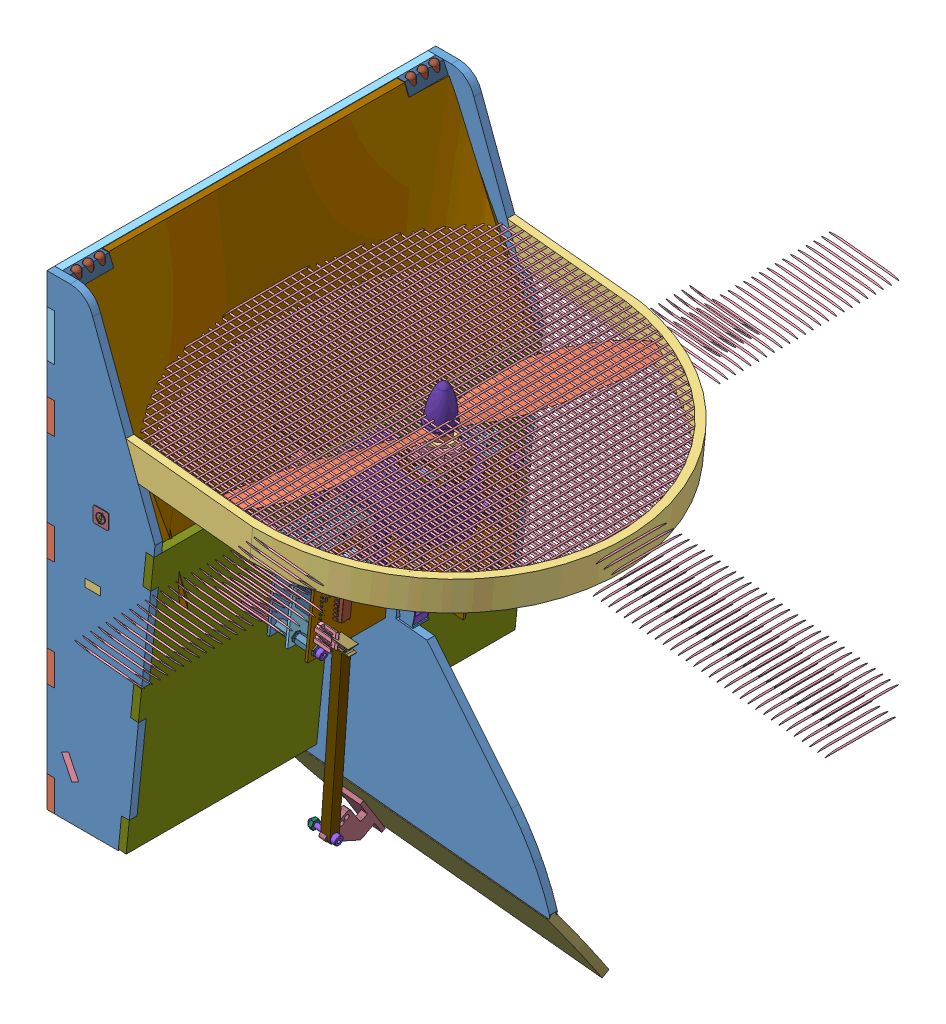
SolidWorks assembly AssTotaleSimu7, configuration Défaut. Lengths in mm.
Overall size (253.25 382.9 251.6).
1779 component instances, 238 part files, 11 mates.
Components (placement in the parent):
- AssStructSimu-1: AssStructSimu [Défaut] at (-125.7658 -1.8483 624.6548) x (1 0 0) z (0 0 -1) size (253.25 324.59 251.6)
  - AssBase-1: AssBase [Défaut] at (36.5482 -71.0398 34.0612) size (86.08 302.3 251.6)
    - AssD-1: AssD [Défaut] at (39.0992 31.0201 8.5) size (69.5 300 22)
      - P1-1: P1 [Défaut] at (-95.5819 194.6656 377.5) size (69.5 300 5)
      - P5-1: P5 [Défaut] at (-100.5819 -35.3344 360.5) x (0 1 0) z (1 0 0) size (230 22 5)
    - AssG-1: AssG [Défaut] at (39.0992 31.0201 -236.5) size (69.5 300 22)
      - P1-1: P1 [Défaut] at (-95.5819 194.6656 377.5) size (69.5 300 5)
      - P5-1: P5 [Défaut] at (-95.5819 -35.3344 399.5) x (0 1 0) z (-1 0 0) size (230 22 5)
    - P7-1: P7 [Défaut] at (-1.4828 89.6857 370.5) x (0 0 -1) z (0 -1 0) size (250 54.5 5)
    - P4-1: P4 [Défaut] at (-63.2363 165.9323 386) x (0 0 -1) z (0.898794 -0.438371 0) size (250 60.5 66.27)
    - P3-1: P3 [Défaut] at (-56.4828 -74.3143 146) x (0 0 1) z (-1 0 0) size (250 70 5)
    - P4b-1: P4b [Défaut] at (-58.7423 163.7404 190) x (0 0 1) z (0.438371 0.898794 0) size (152 56 2)
    - battery-1: battery [Défaut] at (-39.0156 204.1861 197.5) x (0 0 1) z (0.898794 -0.438371 0) size (137 43 30)
    - socket head cap screw 4762_din-1: socket head cap screw 4762_din [EN ISO 4762 M3 x 10 - 10N] at (-27.7008 145.2627 193) x (0.438371 0.898794 0) z (0 0 -1) size (13 5.5 5.5)
    - socket head cap screw 4762_din-2: socket head cap screw 4762_din [EN ISO 4762 M3 x 10 - 10N] at (-27.7008 145.2627 339) x (0.438371 0.898794 0) z (-0.791285 0.385936 -0.474259) size (13 5.5 5.5)
    - socket head cap screw 4762_din-3: socket head cap screw 4762_din [EN ISO 4762 M3 x 10 - 10N] at (-42.0815 152.2766 339) x (0.438371 0.898794 0) z (-0.001489 0.000726 -0.999999) size (13 5.5 5.5)
    - socket head cap screw 4762_din-4: socket head cap screw 4762_din [EN ISO 4762 M3 x 10 - 10N] at (-42.0815 152.2766 193) x (0.438371 0.898794 0) z (-0.031331 0.015281 -0.999392) size (13 5.5 5.5)
    - P11-1: P11 [Défaut] at (-57.5734 -73.9703 146.7843) x (0.005072 0 0.999987) z (0.006197 0.999981 -0.000031) size (240 65 164)
    - AssPhare-1: AssPhare [Défaut] at (-52.8518 -67.6977 411) x (0 1 0) z (0 0 -1) size (35.8 8 25)
      - piece_led-1: piece_led [Défaut] at (-6.6166 -3.631 25) size (7 8 25)
      - LED 5mm-1: LED 5mm [Valor predeterminado] at (-0.1166 0.369 30) x (0 0 1) z (-1 0 0) size (10.06 6 40.8)
      - LED 5mm-2: LED 5mm [Valor predeterminado] at (-0.1166 0.369 37.5) x (0 0 1) z (-1 0 0) size (10.06 6 40.8)
      - LED 5mm-3: LED 5mm [Valor predeterminado] at (-0.1166 0.369 45) x (0 0 1) z (-1 0 0) size (10.06 6 40.8)
    - AssPhare-2: AssPhare [Défaut] at (-52.8518 -67.6977 196) x (0 1 0) z (0 0 -1) size (35.8 8 25)
      - piece_led-1: piece_led [Défaut] at (-6.6166 -3.631 25) size (7 8 25)
      - LED 5mm-1: LED 5mm [Valor predeterminado] at (-0.1166 0.369 30) x (0 0 1) z (-1 0 0) size (10.06 6 40.8)
      - LED 5mm-2: LED 5mm [Valor predeterminado] at (-0.1166 0.369 37.5) x (0 0 1) z (-1 0 0) size (10.06 6 40.8)
      - LED 5mm-3: LED 5mm [Valor predeterminado] at (-0.1166 0.369 45) x (0 0 1) z (-1 0 0) size (10.06 6 40.8)
    - AssLogo-1: AssLogo [Défaut] at (-27.8835 45.1673 148.1054) x (-1 0 0) z (0 0 -1) size (10 10 0.8)
      - logo1-1: logo1 [Défaut] at (-6.5271 -4.4734 6.5054) size (5.8 7.71 0.4)
      - logo2-1: logo2 [Défaut] at (-6.4007 -4.4815 7.1054) size (10 10 0.4)
    - AssLogo-2: AssLogo [Défaut] at (-25.082 45.1673 383.8946) size (10 10 0.8)
      - logo1-1: logo1 [Défaut] at (-6.5271 -4.4734 6.5054) size (5.8 7.71 0.4)
      - logo2-1: logo2 [Défaut] at (-6.4007 -4.4815 7.1054) size (10 10 0.4)
    - support2-1: support2 [Défaut] at (-61.5648 191.7124 276) x (-0.017452 -0.999848 0) z (0.999848 -0.017452 0) size (75 20 10)
    - socket head cap screw 4762_din-5: socket head cap screw 4762_din [EN ISO 4762 M3 x 5 - 5N] at (-61.652 186.7132 269.3333) x (0.999848 -0.017452 0) z (-0.002158 -0.123615 0.992328) size (8 5.5 5.5)
    - socket head cap screw 4762_din-6: socket head cap screw 4762_din [EN ISO 4762 M3 x 5 - 5N] at (-61.652 186.7132 262.6667) x (0.999848 -0.017452 0) z (0 0 1) size (8 5.5 5.5)
    - socket head cap screw 4762_din-7: socket head cap screw 4762_din [EN ISO 4762 M3 x 25 - 18N] at (-55.2963 121.0922 253) x (0 0 1) z (-1 0 0) size (28 5.5 5.5)
    - hex nut style 1 gradeab_din-1: hex nut style 1 gradeab_din [Hexagon Nut ISO 4032 - M3 - W - N] at (-55.2963 121.0922 276) x (-0.923728 -0.383049 0) z (0 0 -1) size (5.5 6.35 2.4)
  - AssToitMot-1: AssToitMot [Défaut] at (-168.5238 43.6961 238.494) x (0 0 -1) z (0.9948 0.101852 0) size (250 207.5 205)
    - AssToit-1: AssToit [Défaut] at (-23.0702 -16.5789 -3.7148) size (250 207.5 205)
      - P8-1: P8 [Défaut] at (-38.4971 122.5921 203.5) size (250 175 5)
      - P12-1: P12 [Défaut] at (-60.4971 -63.4079 265.5) x (1 0 0) z (0 -1 0) size (44.28 76.64 55)
      - P13-1: P13 [Défaut] at (-35.9971 -52.8579 208.5) x (0 0 1) z (-1 0 0) size (64 15.55 5)
      - P10_2-1: P10_2 [Défaut] at (-35.9971 111.5921 171) x (0 0 1) z (-1 0 0) size (188.5 117.6 5)
    - Parallax-Servo_DUMMY-1: Parallax-Servo_DUMMY [Défaut] at (-61.6002 -51.5207 216.6662) x (1 0 0) z (0 1 0) size (20.07 42.67 55.64)
    - socket head cap screw 4762_din-1: socket head cap screw 4762_din [EN ISO 4762 M2.5 x 5 - 5N] at (-51.9272 -76.4868 259.2852) x (0 -1 0) z (-0.546944 0 0.837169) size (7.5 4.5 4.5)
    - socket head cap screw 4762_din-2: socket head cap screw 4762_din [EN ISO 4762 M2.5 x 5 - 5N] at (-61.5672 -76.4868 268.9252) x (0 -1 0) z (-0.546944 0 0.837169) size (7.5 4.5 4.5)
    - socket head cap screw 4762_din-3: socket head cap screw 4762_din [EN ISO 4762 M2.5 x 5 - 5N] at (-71.2072 -76.4868 259.2852) x (0 -1 0) z (-0.546944 0 0.837169) size (7.5 4.5 4.5)
    - socket head cap screw 4762_din-4: socket head cap screw 4762_din [EN ISO 4762 M2.5 x 5 - 5N] at (-61.5672 -76.4868 249.6452) x (0 -1 0) z (-0.546944 0 0.837169) size (7.5 4.5 4.5)
    - AssPhare-1: AssPhare [Défaut] at (8.4328 83.3966 196.1542) x (0 -1 0) z (1 0 0) size (35.8 8 25)
      - piece_led-1: piece_led [Défaut] at (-6.6166 -3.631 25) size (7 8 25)
      - LED 5mm-1: LED 5mm [Valor predeterminado] at (-0.1166 0.369 30) x (0 0 1) z (-1 0 0) size (10.06 6 40.8)
      - LED 5mm-2: LED 5mm [Valor predeterminado] at (-0.1166 0.369 37.5) x (0 0 1) z (-1 0 0) size (10.06 6 40.8)
      - LED 5mm-3: LED 5mm [Valor predeterminado] at (-0.1166 0.369 45) x (0 0 1) z (-1 0 0) size (10.06 6 40.8)
    - AssPhare-2: AssPhare [Défaut] at (-206.5672 83.3966 196.1542) x (0 -1 0) z (1 0 0) size (35.8 8 25)
      - piece_led-1: piece_led [Défaut] at (-6.6166 -3.631 25) size (7 8 25)
      - LED 5mm-1: LED 5mm [Valor predeterminado] at (-0.1166 0.369 30) x (0 0 1) z (-1 0 0) size (10.06 6 40.8)
      - LED 5mm-2: LED 5mm [Valor predeterminado] at (-0.1166 0.369 37.5) x (0 0 1) z (-1 0 0) size (10.06 6 40.8)
      - LED 5mm-3: LED 5mm [Valor predeterminado] at (-0.1166 0.369 45) x (0 0 1) z (-1 0 0) size (10.06 6 40.8)
    - socket head cap screw 4762_din-5: socket head cap screw 4762_din [EN ISO 4762 M3 x 10 - 10N] at (-67.0672 -22.9368 210.2852) x (0 0 -1) z (1 0 0) size (13 5.5 5.5)
    - socket head cap screw 4762_din-6: socket head cap screw 4762_din [EN ISO 4762 M3 x 10 - 10N] at (-56.0672 -72.9868 210.2852) x (0 0 -1) z (1 0 0) size (13 5.5 5.5)
    - socket head cap screw 4762_din-7: socket head cap screw 4762_din [EN ISO 4762 M3 x 10 - 10N] at (-67.0672 -72.9868 210.2852) x (0 0 -1) z (1 0 0) size (13 5.5 5.5)
    - socket head cap screw 4762_din-8: socket head cap screw 4762_din [EN ISO 4762 M3 x 10 - 10N] at (-56.0672 -22.9368 210.2852) x (0 0 -1) z (1 0 0) size (13 5.5 5.5)
    - hex nut style 1 gradeab_din-1: hex nut style 1 gradeab_din [Hexagon Nut ISO 4032 - M3 - W - N] at (-67.0672 -72.9868 197.3852) x (-0.923728 -0.383049 0) z (0 0 -1) size (5.5 6.35 2.4)
    - hex nut style 1 gradeab_din-2: hex nut style 1 gradeab_din [Hexagon Nut ISO 4032 - M3 - W - N] at (-56.0672 -72.9868 199.7852) size (5.5 6.35 2.4)
    - hex nut style 1 gradeab_din-3: hex nut style 1 gradeab_din [Hexagon Nut ISO 4032 - M3 - W - N] at (-67.0672 -22.9368 199.7852) size (5.5 6.35 2.4)
    - hex nut style 1 gradeab_din-4: hex nut style 1 gradeab_din [Hexagon Nut ISO 4032 - M3 - W - N] at (-56.0672 -22.9368 199.7852) size (5.5 6.35 2.4)
  - AssProtec-1: AssProtec [Défaut] at (86.6746 190.4649 284.6351) x (0 0 -1) z (0.101852 -0.9948 0) size (250 237.46 20)
    - protec3c-1: protec3c [Défaut] at (-140.4261 -87.7568 240) size (250 197 20)
    - AssGrillage-1: AssGrillage [Défaut] at (-370.4609 -132.5428 258.3161) x (0 0 -1) z (1 0 0) size (2.02 237.05 250)
      - barreau-1: barreau [Défaut] at (-1.1839 0.254 200) size (1 1 400)
      - barreau-3: barreau [Défaut] at (-1.1839 5.254 200) size (1 1 400)
      - barreau-4: barreau [Défaut] at (-1.1839 10.254 200) size (1 1 400)
      - barreau-5: barreau [Défaut] at (-1.1839 15.254 200) size (1 1 400)
      - barreau-6: barreau [Défaut] at (-1.1839 20.254 200) size (1 1 400)
      - barreau-7: barreau [Défaut] at (-1.1839 25.254 200) size (1 1 400)
      - barreau-8: barreau [Défaut] at (-1.1839 30.254 200) size (1 1 400)
      - barreau-9: barreau [Défaut] at (-1.1839 35.254 200) size (1 1 400)
      - barreau-10: barreau [Défaut] at (-1.1839 40.254 200) size (1 1 400)
      - barreau-11: barreau [Défaut] at (-1.1839 45.254 200) size (1 1 400)
      - barreau-12: barreau [Défaut] at (-1.1839 50.254 200) size (1 1 400)
      - barreau-13: barreau [Défaut] at (-1.1839 55.254 200) size (1 1 400)
      - barreau-14: barreau [Défaut] at (-1.1839 60.254 200) size (1 1 400)
      - barreau-15: barreau [Défaut] at (-1.1839 65.254 200) size (1 1 400)
      - barreau-16: barreau [Défaut] at (-1.1839 70.254 200) size (1 1 400)
      - barreau-17: barreau [Défaut] at (-1.1839 75.254 200) size (1 1 400)
      - barreau-18: barreau [Défaut] at (-1.1839 80.254 200) size (1 1 400)
      - barreau-19: barreau [Défaut] at (-1.1839 85.254 200) size (1 1 400)
      - barreau-20: barreau [Défaut] at (-1.1839 90.254 200) size (1 1 400)
      - barreau-21: barreau [Défaut] at (-1.1839 95.254 200) size (1 1 400)
      - barreau-22: barreau [Défaut] at (-1.1839 100.254 200) size (1 1 400)
      - barreau-23: barreau [Défaut] at (-1.1839 105.254 200) size (1 1 400)
      - barreau-24: barreau [Défaut] at (-1.1839 110.254 200) size (1 1 400)
      - barreau-25: barreau [Défaut] at (-1.1839 115.254 200) size (1 1 400)
      - barreau-26: barreau [Défaut] at (-1.1839 120.254 200) size (1 1 400)
      - barreau-27: barreau [Défaut] at (-1.1839 125.254 200) size (1 1 400)
      - barreau-28: barreau [Défaut] at (-1.1839 130.254 200) size (1 1 400)
      - barreau-29: barreau [Défaut] at (-1.1839 135.254 200) size (1 1 400)
      - barreau-30: barreau [Défaut] at (-1.1839 140.254 200) size (1 1 400)
      - barreau-31: barreau [Défaut] at (-1.1839 145.254 200) size (1 1 400)
      - barreau-32: barreau [Défaut] at (-1.1839 150.254 200) size (1 1 400)
      - barreau-33: barreau [Défaut] at (-1.1839 155.254 200) size (1 1 400)
      - barreau-34: barreau [Défaut] at (-1.1839 160.254 200) size (1 1 400)
      - barreau-35: barreau [Défaut] at (-1.1839 165.254 200) size (1 1 400)
      - barreau-36: barreau [Défaut] at (-1.1839 170.254 200) size (1 1 400)
      - barreau-37: barreau [Défaut] at (-1.1839 175.254 200) size (1 1 400)
      - barreau-38: barreau [Défaut] at (-1.1839 180.254 200) size (1 1 400)
      - barreau-39: barreau [Défaut] at (-1.1839 185.254 200) size (1 1 400)
      - barreau-40: barreau [Défaut] at (-1.1839 190.254 200) size (1 1 400)
      - barreau-41: barreau [Défaut] at (-1.1839 195.254 200) size (1 1 400)
      - barreau-42: barreau [Défaut] at (-0.1839 -1.5314 598.7823) x (0.998922 0 0.04641) z (0 1 0) size (1 1 400)
      - barreau-43: barreau [Défaut] at (-1.1839 200.254 200) size (1 1 400)
      - barreau-44: barreau [Défaut] at (-1.1839 205.254 200) size (1 1 400)
      - barreau-45: barreau [Défaut] at (-1.1839 210.254 200) size (1 1 400)
      - barreau-46: barreau [Défaut] at (-1.1839 215.254 200) size (1 1 400)
      - barreau-47: barreau [Défaut] at (-1.1839 220.254 200) size (1 1 400)
      - barreau-48: barreau [Défaut] at (-1.1839 225.254 200) size (1 1 400)
      - barreau-49: barreau [Défaut] at (-1.1839 230.254 200) size (1 1 400)
      - barreau-50: barreau [Défaut] at (-1.1839 235.254 200) size (1 1 400)
      - barreau-51: barreau [Défaut] at (-1.1839 240.254 200) size (1 1 400)
      - barreau-52: barreau [Défaut] at (-1.1839 245.254 200) size (1 1 400)
      - barreau-53: barreau [Défaut] at (-1.1839 250.254 200) size (1 1 400)
      - barreau-54: barreau [Défaut] at (-1.1839 255.254 200) size (1 1 400)
      - barreau-55: barreau [Défaut] at (-1.1839 260.254 200) size (1 1 400)
      - barreau-56: barreau [Défaut] at (-1.1839 265.254 200) size (1 1 400)
      - barreau-57: barreau [Défaut] at (-1.1839 270.254 200) size (1 1 400)
      - barreau-58: barreau [Défaut] at (-1.1839 275.254 200) size (1 1 400)
      - barreau-59: barreau [Défaut] at (-1.1839 280.254 200) size (1 1 400)
      - barreau-60: barreau [Défaut] at (-1.1839 285.254 200) size (1 1 400)
      - barreau-61: barreau [Défaut] at (-1.1839 290.254 200) size (1 1 400)
      - barreau-62: barreau [Défaut] at (-1.1839 295.254 200) size (1 1 400)
      - barreau-63: barreau [Défaut] at (-1.1839 300.254 200) size (1 1 400)
      - barreau-64: barreau [Défaut] at (-1.1839 305.254 200) size (1 1 400)
      - barreau-65: barreau [Défaut] at (-1.1839 310.254 200) size (1 1 400)
      - barreau-66: barreau [Défaut] at (-1.1839 315.254 200) size (1 1 400)
      - barreau-67: barreau [Défaut] at (-1.1839 320.254 200) size (1 1 400)
      - barreau-68: barreau [Défaut] at (-1.1839 325.254 200) size (1 1 400)
      - barreau-69: barreau [Défaut] at (-1.1839 330.254 200) size (1 1 400)
      - barreau-70: barreau [Défaut] at (-1.1839 335.254 200) size (1 1 400)
      - barreau-71: barreau [Défaut] at (-1.1839 340.254 200) size (1 1 400)
      - barreau-72: barreau [Défaut] at (-1.1839 345.254 200) size (1 1 400)
      - barreau-73: barreau [Défaut] at (-1.1839 350.254 200) size (1 1 400)
      - barreau-74: barreau [Défaut] at (-1.1839 355.254 200) size (1 1 400)
      - barreau-75: barreau [Défaut] at (-1.1839 360.254 200) size (1 1 400)
      - barreau-76: barreau [Défaut] at (-1.1839 365.254 200) size (1 1 400)
      - barreau-77: barreau [Défaut] at (-1.1839 370.254 200) size (1 1 400)
      - barreau-78: barreau [Défaut] at (-1.1839 375.254 200) size (1 1 400)
      - barreau-79: barreau [Défaut] at (-1.1839 380.254 200) size (1 1 400)
      - barreau-80: barreau [Défaut] at (-1.1839 385.254 200) size (1 1 400)
      - barreau-81: barreau [Défaut] at (-1.1839 390.254 200) size (1 1 400)
      - barreau-82: barreau [Défaut] at (-1.1839 395.254 200) size (1 1 400)
      - barreau-136: barreau [Défaut] at (-0.1839 -1.5314 593.7823) x (0.998922 0 0.04641) z (0 1 0) size (1 1 400)
      - barreau-137: barreau [Défaut] at (-0.1839 -1.5314 588.7823) x (0.998922 0 0.04641) z (0 1 0) size (1 1 400)
      - barreau-138: barreau [Défaut] at (-0.1839 -1.5314 583.7823) x (0.998922 0 0.04641) z (0 1 0) size (1 1 400)
      - barreau-139: barreau [Défaut] at (-0.1839 -1.5314 578.7823) x (0.998922 0 0.04641) z (0 1 0) size (1 1 400)
      - barreau-140: barreau [Défaut] at (-0.1839 -1.5314 573.7823) x (0.998922 0 0.04641) z (0 1 0) size (1 1 400)
      - barreau-141: barreau [Défaut] at (-0.1839 -1.5314 568.7823) x (0.998922 0 0.04641) z (0 1 0) size (1 1 400)
      - barreau-142: barreau [Défaut] at (-0.1839 -1.5314 563.7823) x (0.998922 0 0.04641) z (0 1 0) size (1 1 400)
      - barreau-143: barreau [Défaut] at (-0.1839 -1.5314 558.7823) x (0.998922 0 0.04641) z (0 1 0) size (1 1 400)
      - barreau-144: barreau [Défaut] at (-0.1839 -1.5314 553.7823) x (0.998922 0 0.04641) z (0 1 0) size (1 1 400)
      - barreau-145: barreau [Défaut] at (-0.1839 -1.5314 548.7823) x (0.998922 0 0.04641) z (0 1 0) size (1 1 400)
      - barreau-146: barreau [Défaut] at (-0.1839 -1.5314 543.7823) x (0.998922 0 0.04641) z (0 1 0) size (1 1 400)
      - barreau-147: barreau [Défaut] at (-0.1839 -1.5314 538.7823) x (0.998922 0 0.04641) z (0 1 0) size (1 1 400)
      - barreau-148: barreau [Défaut] at (-0.1839 -1.5314 533.7823) x (0.998922 0 0.04641) z (0 1 0) size (1 1 400)
      - barreau-149: barreau [Défaut] at (-0.1839 -1.5314 528.7823) x (0.998922 0 0.04641) z (0 1 0) size (1 1 400)
      - barreau-150: barreau [Défaut] at (-0.1839 -1.5314 523.7823) x (0.998922 0 0.04641) z (0 1 0) size (1 1 400)
      - barreau-151: barreau [Défaut] at (-0.1839 -1.5314 518.7823) x (0.998922 0 0.04641) z (0 1 0) size (1 1 400)
      - barreau-152: barreau [Défaut] at (-0.1839 -1.5314 513.7823) x (0.998922 0 0.04641) z (0 1 0) size (1 1 400)
      - barreau-153: barreau [Défaut] at (-0.1839 -1.5314 508.7823) x (0.998922 0 0.04641) z (0 1 0) size (1 1 400)
      - barreau-154: barreau [Défaut] at (-0.1839 -1.5314 503.7823) x (0.998922 0 0.04641) z (0 1 0) size (1 1 400)
      - barreau-155: barreau [Défaut] at (-0.1839 -1.5314 498.7823) x (0.998922 0 0.04641) z (0 1 0) size (1 1 400)
      - barreau-156: barreau [Défaut] at (-0.1839 -1.5314 493.7823) x (0.998922 0 0.04641) z (0 1 0) size (1 1 400)
      - barreau-157: barreau [Défaut] at (-0.1839 -1.5314 488.7823) x (0.998922 0 0.04641) z (0 1 0) size (1 1 400)
      - barreau-158: barreau [Défaut] at (-0.1839 -1.5314 483.7823) x (0.998922 0 0.04641) z (0 1 0) size (1 1 400)
      - barreau-159: barreau [Défaut] at (-0.1839 -1.5314 478.7823) x (0.998922 0 0.04641) z (0 1 0) size (1 1 400)
      - barreau-160: barreau [Défaut] at (-0.1839 -1.5314 473.7823) x (0.998922 0 0.04641) z (0 1 0) size (1 1 400)
      - barreau-161: barreau [Défaut] at (-0.1839 -1.5314 468.7823) x (0.998922 0 0.04641) z (0 1 0) size (1 1 400)
      - barreau-162: barreau [Défaut] at (-0.1839 -1.5314 463.7823) x (0.998922 0 0.04641) z (0 1 0) size (1 1 400)
      - barreau-163: barreau [Défaut] at (-0.1839 -1.5314 458.7823) x (0.998922 0 0.04641) z (0 1 0) size (1 1 400)
      - barreau-164: barreau [Défaut] at (-0.1839 -1.5314 453.7823) x (0.998922 0 0.04641) z (0 1 0) size (1 1 400)
      - barreau-165: barreau [Défaut] at (-0.1839 -1.5314 448.7823) x (0.998922 0 0.04641) z (0 1 0) size (1 1 400)
      - barreau-166: barreau [Défaut] at (-0.1839 -1.5314 443.7823) x (0.998922 0 0.04641) z (0 1 0) size (1 1 400)
      - barreau-167: barreau [Défaut] at (-0.1839 -1.5314 438.7823) x (0.998922 0 0.04641) z (0 1 0) size (1 1 400)
      - barreau-168: barreau [Défaut] at (-0.1839 -1.5314 433.7823) x (0.998922 0 0.04641) z (0 1 0) size (1 1 400)
      - barreau-169: barreau [Défaut] at (-0.1839 -1.5314 428.7823) x (0.998922 0 0.04641) z (0 1 0) size (1 1 400)
      - barreau-170: barreau [Défaut] at (-0.1839 -1.5314 423.7823) x (0.998922 0 0.04641) z (0 1 0) size (1 1 400)
      - barreau-171: barreau [Défaut] at (-0.1839 -1.5314 418.7823) x (0.998922 0 0.04641) z (0 1 0) size (1 1 400)
      - barreau-172: barreau [Défaut] at (-0.1839 -1.5314 413.7823) x (0.998922 0 0.04641) z (0 1 0) size (1 1 400)
      - barreau-173: barreau [Défaut] at (-0.1839 -1.5314 408.7823) x (0.998922 0 0.04641) z (0 1 0) size (1 1 400)
      - barreau-174: barreau [Défaut] at (-0.1839 -1.5314 403.7823) x (0.998922 0 0.04641) z (0 1 0) size (1 1 400)
      - barreau-175: barreau [Défaut] at (-0.1839 -1.5314 398.7823) x (0.998922 0 0.04641) z (0 1 0) size (1 1 400)
      - barreau-176: barreau [Défaut] at (-0.1839 -1.5314 393.7823) x (0.998922 0 0.04641) z (0 1 0) size (1 1 400)
      - barreau-177: barreau [Défaut] at (-0.1839 -1.5314 388.7823) x (0.998922 0 0.04641) z (0 1 0) size (1 1 400)
      - barreau-178: barreau [Défaut] at (-0.1839 -1.5314 383.7823) x (0.998922 0 0.04641) z (0 1 0) size (1 1 400)
      - barreau-179: barreau [Défaut] at (-0.1839 -1.5314 378.7823) x (0.998922 0 0.04641) z (0 1 0) size (1 1 400)
      - barreau-180: barreau [Défaut] at (-0.1839 -1.5314 373.7823) x (0.998922 0 0.04641) z (0 1 0) size (1 1 400)
      - barreau-181: barreau [Défaut] at (-0.1839 -1.5314 368.7823) x (0.998922 0 0.04641) z (0 1 0) size (1 1 400)
      - barreau-182: barreau [Défaut] at (-0.1839 -1.5314 363.7823) x (0.998922 0 0.04641) z (0 1 0) size (1 1 400)
      - barreau-183: barreau [Défaut] at (-0.1839 -1.5314 358.7823) x (0.998922 0 0.04641) z (0 1 0) size (1 1 400)
      - barreau-184: barreau [Défaut] at (-0.1839 -1.5314 353.7823) x (0.998922 0 0.04641) z (0 1 0) size (1 1 400)
      - barreau-185: barreau [Défaut] at (-0.1839 -1.5314 348.7823) x (0.998922 0 0.04641) z (0 1 0) size (1 1 400)
      - barreau-186: barreau [Défaut] at (-0.1839 -1.5314 343.7823) x (0.998922 0 0.04641) z (0 1 0) size (1 1 400)
      - barreau-187: barreau [Défaut] at (-0.1839 -1.5314 338.7823) x (0.998922 0 0.04641) z (0 1 0) size (1 1 400)
      - barreau-188: barreau [Défaut] at (-0.1839 -1.5314 333.7823) x (0.998922 0 0.04641) z (0 1 0) size (1 1 400)
      - barreau-189: barreau [Défaut] at (-0.1839 -1.5314 328.7823) x (0.998922 0 0.04641) z (0 1 0) size (1 1 400)
      - barreau-190: barreau [Défaut] at (-0.1839 -1.5314 323.7823) x (0.998922 0 0.04641) z (0 1 0) size (1 1 400)
      - barreau-191: barreau [Défaut] at (-0.1839 -1.5314 318.7823) x (0.998922 0 0.04641) z (0 1 0) size (1 1 400)
      - barreau-192: barreau [Défaut] at (-0.1839 -1.5314 313.7823) x (0.998922 0 0.04641) z (0 1 0) size (1 1 400)
      - barreau-193: barreau [Défaut] at (-0.1839 -1.5314 308.7823) x (0.998922 0 0.04641) z (0 1 0) size (1 1 400)
      - barreau-194: barreau [Défaut] at (-0.1839 -1.5314 303.7823) x (0.998922 0 0.04641) z (0 1 0) size (1 1 400)
      - barreau-195: barreau [Défaut] at (-0.1839 -1.5314 298.7823) x (0.998922 0 0.04641) z (0 1 0) size (1 1 400)
      - barreau-196: barreau [Défaut] at (-0.1839 -1.5314 293.7823) x (0.998922 0 0.04641) z (0 1 0) size (1 1 400)
      - barreau-197: barreau [Défaut] at (-0.1839 -1.5314 288.7823) x (0.998922 0 0.04641) z (0 1 0) size (1 1 400)
      - barreau-198: barreau [Défaut] at (-0.1839 -1.5314 283.7823) x (0.998922 0 0.04641) z (0 1 0) size (1 1 400)
      - barreau-199: barreau [Défaut] at (-0.1839 -1.5314 278.7823) x (0.998922 0 0.04641) z (0 1 0) size (1 1 400)
      - barreau-200: barreau [Défaut] at (-0.1839 -1.5314 273.7823) x (0.998922 0 0.04641) z (0 1 0) size (1 1 400)
      - barreau-201: barreau [Défaut] at (-0.1839 -1.5314 268.7823) x (0.998922 0 0.04641) z (0 1 0) size (1 1 400)
      - barreau-202: barreau [Défaut] at (-0.1839 -1.5314 263.7823) x (0.998922 0 0.04641) z (0 1 0) size (1 1 400)
      - barreau-203: barreau [Défaut] at (-0.1839 -1.5314 258.7823) x (0.998922 0 0.04641) z (0 1 0) size (1 1 400)
      - barreau-204: barreau [Défaut] at (-0.1839 -1.5314 253.7823) x (0.998922 0 0.04641) z (0 1 0) size (1 1 400)
      - barreau-205: barreau [Défaut] at (-0.1839 -1.5314 248.7823) x (0.998922 0 0.04641) z (0 1 0) size (1 1 400)
      - barreau-206: barreau [Défaut] at (-0.1839 -1.5314 243.7823) x (0.998922 0 0.04641) z (0 1 0) size (1 1 400)
      - barreau-207: barreau [Défaut] at (-0.1839 -1.5314 238.7823) x (0.998922 0 0.04641) z (0 1 0) size (1 1 400)
      - barreau-208: barreau [Défaut] at (-0.1839 -1.5314 233.7823) x (0.998922 0 0.04641) z (0 1 0) size (1 1 400)
      - barreau-209: barreau [Défaut] at (-0.1839 -1.5314 228.7823) x (0.998922 0 0.04641) z (0 1 0) size (1 1 400)
      - barreau-210: barreau [Défaut] at (-0.1839 -1.5314 223.7823) x (0.998922 0 0.04641) z (0 1 0) size (1 1 400)
      - barreau-211: barreau [Défaut] at (-0.1839 -1.5314 218.7823) x (0.998922 0 0.04641) z (0 1 0) size (1 1 400)
      - barreau-212: barreau [Défaut] at (-0.1839 -1.5314 213.7823) x (0.998922 0 0.04641) z (0 1 0) size (1 1 400)
      - barreau-213: barreau [Défaut] at (-0.1839 -1.5314 208.7823) x (0.998922 0 0.04641) z (0 1 0) size (1 1 400)
      - barreau-214: barreau [Défaut] at (-0.1839 -1.5314 203.7823) x (0.998922 0 0.04641) z (0 1 0) size (1 1 400)
    - AssGrillage-2: AssGrillage [Défaut] at (339.6086 -132.5428 241.6839) x (0 0 1) z (-1 0 0) size (2.02 237.05 250)
      - barreau-1: barreau [Défaut] at (-1.1839 0.254 200) size (1 1 400)
      - barreau-3: barreau [Défaut] at (-1.1839 5.254 200) size (1 1 400)
      - barreau-4: barreau [Défaut] at (-1.1839 10.254 200) size (1 1 400)
      - barreau-5: barreau [Défaut] at (-1.1839 15.254 200) size (1 1 400)
      - barreau-6: barreau [Défaut] at (-1.1839 20.254 200) size (1 1 400)
      - barreau-7: barreau [Défaut] at (-1.1839 25.254 200) size (1 1 400)
      - barreau-8: barreau [Défaut] at (-1.1839 30.254 200) size (1 1 400)
      - barreau-9: barreau [Défaut] at (-1.1839 35.254 200) size (1 1 400)
      - barreau-10: barreau [Défaut] at (-1.1839 40.254 200) size (1 1 400)
      - barreau-11: barreau [Défaut] at (-1.1839 45.254 200) size (1 1 400)
      - barreau-12: barreau [Défaut] at (-1.1839 50.254 200) size (1 1 400)
      - barreau-13: barreau [Défaut] at (-1.1839 55.254 200) size (1 1 400)
      - barreau-14: barreau [Défaut] at (-1.1839 60.254 200) size (1 1 400)
      - barreau-15: barreau [Défaut] at (-1.1839 65.254 200) size (1 1 400)
      - barreau-16: barreau [Défaut] at (-1.1839 70.254 200) size (1 1 400)
      - barreau-17: barreau [Défaut] at (-1.1839 75.254 200) size (1 1 400)
      - barreau-18: barreau [Défaut] at (-1.1839 80.254 200) size (1 1 400)
      - barreau-19: barreau [Défaut] at (-1.1839 85.254 200) size (1 1 400)
      - barreau-20: barreau [Défaut] at (-1.1839 90.254 200) size (1 1 400)
      - barreau-21: barreau [Défaut] at (-1.1839 95.254 200) size (1 1 400)
      - barreau-22: barreau [Défaut] at (-1.1839 100.254 200) size (1 1 400)
      - barreau-23: barreau [Défaut] at (-1.1839 105.254 200) size (1 1 400)
      - barreau-24: barreau [Défaut] at (-1.1839 110.254 200) size (1 1 400)
      - barreau-25: barreau [Défaut] at (-1.1839 115.254 200) size (1 1 400)
      - barreau-26: barreau [Défaut] at (-1.1839 120.254 200) size (1 1 400)
      - barreau-27: barreau [Défaut] at (-1.1839 125.254 200) size (1 1 400)
      - barreau-28: barreau [Défaut] at (-1.1839 130.254 200) size (1 1 400)
      - barreau-29: barreau [Défaut] at (-1.1839 135.254 200) size (1 1 400)
      - barreau-30: barreau [Défaut] at (-1.1839 140.254 200) size (1 1 400)
      - barreau-31: barreau [Défaut] at (-1.1839 145.254 200) size (1 1 400)
      - barreau-32: barreau [Défaut] at (-1.1839 150.254 200) size (1 1 400)
      - barreau-33: barreau [Défaut] at (-1.1839 155.254 200) size (1 1 400)
      - barreau-34: barreau [Défaut] at (-1.1839 160.254 200) size (1 1 400)
      - barreau-35: barreau [Défaut] at (-1.1839 165.254 200) size (1 1 400)
      - barreau-36: barreau [Défaut] at (-1.1839 170.254 200) size (1 1 400)
      - barreau-37: barreau [Défaut] at (-1.1839 175.254 200) size (1 1 400)
      - barreau-38: barreau [Défaut] at (-1.1839 180.254 200) size (1 1 400)
      - barreau-39: barreau [Défaut] at (-1.1839 185.254 200) size (1 1 400)
      - barreau-40: barreau [Défaut] at (-1.1839 190.254 200) size (1 1 400)
      - barreau-41: barreau [Défaut] at (-1.1839 195.254 200) size (1 1 400)
      - barreau-42: barreau [Défaut] at (-0.1839 -1.5314 598.7823) x (0.998922 0 0.04641) z (0 1 0) size (1 1 400)
      - barreau-43: barreau [Défaut] at (-1.1839 200.254 200) size (1 1 400)
      - barreau-44: barreau [Défaut] at (-1.1839 205.254 200) size (1 1 400)
      - barreau-45: barreau [Défaut] at (-1.1839 210.254 200) size (1 1 400)
      - barreau-46: barreau [Défaut] at (-1.1839 215.254 200) size (1 1 400)
      - barreau-47: barreau [Défaut] at (-1.1839 220.254 200) size (1 1 400)
      - barreau-48: barreau [Défaut] at (-1.1839 225.254 200) size (1 1 400)
      - barreau-49: barreau [Défaut] at (-1.1839 230.254 200) size (1 1 400)
      - barreau-50: barreau [Défaut] at (-1.1839 235.254 200) size (1 1 400)
      - barreau-51: barreau [Défaut] at (-1.1839 240.254 200) size (1 1 400)
      - barreau-52: barreau [Défaut] at (-1.1839 245.254 200) size (1 1 400)
      - barreau-53: barreau [Défaut] at (-1.1839 250.254 200) size (1 1 400)
      - barreau-54: barreau [Défaut] at (-1.1839 255.254 200) size (1 1 400)
      - barreau-55: barreau [Défaut] at (-1.1839 260.254 200) size (1 1 400)
      - barreau-56: barreau [Défaut] at (-1.1839 265.254 200) size (1 1 400)
      - barreau-57: barreau [Défaut] at (-1.1839 270.254 200) size (1 1 400)
      - barreau-58: barreau [Défaut] at (-1.1839 275.254 200) size (1 1 400)
      - barreau-59: barreau [Défaut] at (-1.1839 280.254 200) size (1 1 400)
      - barreau-60: barreau [Défaut] at (-1.1839 285.254 200) size (1 1 400)
      - barreau-61: barreau [Défaut] at (-1.1839 290.254 200) size (1 1 400)
      - barreau-62: barreau [Défaut] at (-1.1839 295.254 200) size (1 1 400)
      - barreau-63: barreau [Défaut] at (-1.1839 300.254 200) size (1 1 400)
      - barreau-64: barreau [Défaut] at (-1.1839 305.254 200) size (1 1 400)
      - barreau-65: barreau [Défaut] at (-1.1839 310.254 200) size (1 1 400)
      - barreau-66: barreau [Défaut] at (-1.1839 315.254 200) size (1 1 400)
      - barreau-67: barreau [Défaut] at (-1.1839 320.254 200) size (1 1 400)
      - barreau-68: barreau [Défaut] at (-1.1839 325.254 200) size (1 1 400)
      - barreau-69: barreau [Défaut] at (-1.1839 330.254 200) size (1 1 400)
      - barreau-70: barreau [Défaut] at (-1.1839 335.254 200) size (1 1 400)
      - barreau-71: barreau [Défaut] at (-1.1839 340.254 200) size (1 1 400)
      - barreau-72: barreau [Défaut] at (-1.1839 345.254 200) size (1 1 400)
      - barreau-73: barreau [Défaut] at (-1.1839 350.254 200) size (1 1 400)
      - barreau-74: barreau [Défaut] at (-1.1839 355.254 200) size (1 1 400)
      - barreau-75: barreau [Défaut] at (-1.1839 360.254 200) size (1 1 400)
      - barreau-76: barreau [Défaut] at (-1.1839 365.254 200) size (1 1 400)
      - barreau-77: barreau [Défaut] at (-1.1839 370.254 200) size (1 1 400)
      - barreau-78: barreau [Défaut] at (-1.1839 375.254 200) size (1 1 400)
      - barreau-79: barreau [Défaut] at (-1.1839 380.254 200) size (1 1 400)
      - barreau-80: barreau [Défaut] at (-1.1839 385.254 200) size (1 1 400)
      - barreau-81: barreau [Défaut] at (-1.1839 390.254 200) size (1 1 400)
      - barreau-82: barreau [Défaut] at (-1.1839 395.254 200) size (1 1 400)
      - barreau-136: barreau [Défaut] at (-0.1839 -1.5314 593.7823) x (0.998922 0 0.04641) z (0 1 0) size (1 1 400)
      - barreau-137: barreau [Défaut] at (-0.1839 -1.5314 588.7823) x (0.998922 0 0.04641) z (0 1 0) size (1 1 400)
      - barreau-138: barreau [Défaut] at (-0.1839 -1.5314 583.7823) x (0.998922 0 0.04641) z (0 1 0) size (1 1 400)
      - barreau-139: barreau [Défaut] at (-0.1839 -1.5314 578.7823) x (0.998922 0 0.04641) z (0 1 0) size (1 1 400)
      - barreau-140: barreau [Défaut] at (-0.1839 -1.5314 573.7823) x (0.998922 0 0.04641) z (0 1 0) size (1 1 400)
      - barreau-141: barreau [Défaut] at (-0.1839 -1.5314 568.7823) x (0.998922 0 0.04641) z (0 1 0) size (1 1 400)
      - barreau-142: barreau [Défaut] at (-0.1839 -1.5314 563.7823) x (0.998922 0 0.04641) z (0 1 0) size (1 1 400)
      - barreau-143: barreau [Défaut] at (-0.1839 -1.5314 558.7823) x (0.998922 0 0.04641) z (0 1 0) size (1 1 400)
      - barreau-144: barreau [Défaut] at (-0.1839 -1.5314 553.7823) x (0.998922 0 0.04641) z (0 1 0) size (1 1 400)
      - barreau-145: barreau [Défaut] at (-0.1839 -1.5314 548.7823) x (0.998922 0 0.04641) z (0 1 0) size (1 1 400)
      - barreau-146: barreau [Défaut] at (-0.1839 -1.5314 543.7823) x (0.998922 0 0.04641) z (0 1 0) size (1 1 400)
      - barreau-147: barreau [Défaut] at (-0.1839 -1.5314 538.7823) x (0.998922 0 0.04641) z (0 1 0) size (1 1 400)
      - barreau-148: barreau [Défaut] at (-0.1839 -1.5314 533.7823) x (0.998922 0 0.04641) z (0 1 0) size (1 1 400)
      - barreau-149: barreau [Défaut] at (-0.1839 -1.5314 528.7823) x (0.998922 0 0.04641) z (0 1 0) size (1 1 400)
      - barreau-150: barreau [Défaut] at (-0.1839 -1.5314 523.7823) x (0.998922 0 0.04641) z (0 1 0) size (1 1 400)
      - barreau-151: barreau [Défaut] at (-0.1839 -1.5314 518.7823) x (0.998922 0 0.04641) z (0 1 0) size (1 1 400)
      - barreau-152: barreau [Défaut] at (-0.1839 -1.5314 513.7823) x (0.998922 0 0.04641) z (0 1 0) size (1 1 400)
      - barreau-153: barreau [Défaut] at (-0.1839 -1.5314 508.7823) x (0.998922 0 0.04641) z (0 1 0) size (1 1 400)
      - barreau-154: barreau [Défaut] at (-0.1839 -1.5314 503.7823) x (0.998922 0 0.04641) z (0 1 0) size (1 1 400)
      - barreau-155: barreau [Défaut] at (-0.1839 -1.5314 498.7823) x (0.998922 0 0.04641) z (0 1 0) size (1 1 400)
      - barreau-156: barreau [Défaut] at (-0.1839 -1.5314 493.7823) x (0.998922 0 0.04641) z (0 1 0) size (1 1 400)
      - barreau-157: barreau [Défaut] at (-0.1839 -1.5314 488.7823) x (0.998922 0 0.04641) z (0 1 0) size (1 1 400)
      - barreau-158: barreau [Défaut] at (-0.1839 -1.5314 483.7823) x (0.998922 0 0.04641) z (0 1 0) size (1 1 400)
      - barreau-159: barreau [Défaut] at (-0.1839 -1.5314 478.7823) x (0.998922 0 0.04641) z (0 1 0) size (1 1 400)
      - barreau-160: barreau [Défaut] at (-0.1839 -1.5314 473.7823) x (0.998922 0 0.04641) z (0 1 0) size (1 1 400)
      - barreau-161: barreau [Défaut] at (-0.1839 -1.5314 468.7823) x (0.998922 0 0.04641) z (0 1 0) size (1 1 400)
      - barreau-162: barreau [Défaut] at (-0.1839 -1.5314 463.7823) x (0.998922 0 0.04641) z (0 1 0) size (1 1 400)
      - barreau-163: barreau [Défaut] at (-0.1839 -1.5314 458.7823) x (0.998922 0 0.04641) z (0 1 0) size (1 1 400)
      - barreau-164: barreau [Défaut] at (-0.1839 -1.5314 453.7823) x (0.998922 0 0.04641) z (0 1 0) size (1 1 400)
      - barreau-165: barreau [Défaut] at (-0.1839 -1.5314 448.7823) x (0.998922 0 0.04641) z (0 1 0) size (1 1 400)
      - barreau-166: barreau [Défaut] at (-0.1839 -1.5314 443.7823) x (0.998922 0 0.04641) z (0 1 0) size (1 1 400)
      - barreau-167: barreau [Défaut] at (-0.1839 -1.5314 438.7823) x (0.998922 0 0.04641) z (0 1 0) size (1 1 400)
      - barreau-168: barreau [Défaut] at (-0.1839 -1.5314 433.7823) x (0.998922 0 0.04641) z (0 1 0) size (1 1 400)
      - barreau-169: barreau [Défaut] at (-0.1839 -1.5314 428.7823) x (0.998922 0 0.04641) z (0 1 0) size (1 1 400)
      - barreau-170: barreau [Défaut] at (-0.1839 -1.5314 423.7823) x (0.998922 0 0.04641) z (0 1 0) size (1 1 400)
      - barreau-171: barreau [Défaut] at (-0.1839 -1.5314 418.7823) x (0.998922 0 0.04641) z (0 1 0) size (1 1 400)
      - barreau-172: barreau [Défaut] at (-0.1839 -1.5314 413.7823) x (0.998922 0 0.04641) z (0 1 0) size (1 1 400)
      - barreau-173: barreau [Défaut] at (-0.1839 -1.5314 408.7823) x (0.998922 0 0.04641) z (0 1 0) size (1 1 400)
      - barreau-174: barreau [Défaut] at (-0.1839 -1.5314 403.7823) x (0.998922 0 0.04641) z (0 1 0) size (1 1 400)
      - barreau-175: barreau [Défaut] at (-0.1839 -1.5314 398.7823) x (0.998922 0 0.04641) z (0 1 0) size (1 1 400)
      - barreau-176: barreau [Défaut] at (-0.1839 -1.5314 393.7823) x (0.998922 0 0.04641) z (0 1 0) size (1 1 400)
      - barreau-177: barreau [Défaut] at (-0.1839 -1.5314 388.7823) x (0.998922 0 0.04641) z (0 1 0) size (1 1 400)
      - barreau-178: barreau [Défaut] at (-0.1839 -1.5314 383.7823) x (0.998922 0 0.04641) z (0 1 0) size (1 1 400)
      - barreau-179: barreau [Défaut] at (-0.1839 -1.5314 378.7823) x (0.998922 0 0.04641) z (0 1 0) size (1 1 400)
      - barreau-180: barreau [Défaut] at (-0.1839 -1.5314 373.7823) x (0.998922 0 0.04641) z (0 1 0) size (1 1 400)
      - barreau-181: barreau [Défaut] at (-0.1839 -1.5314 368.7823) x (0.998922 0 0.04641) z (0 1 0) size (1 1 400)
      - barreau-182: barreau [Défaut] at (-0.1839 -1.5314 363.7823) x (0.998922 0 0.04641) z (0 1 0) size (1 1 400)
      - barreau-183: barreau [Défaut] at (-0.1839 -1.5314 358.7823) x (0.998922 0 0.04641) z (0 1 0) size (1 1 400)
      - barreau-184: barreau [Défaut] at (-0.1839 -1.5314 353.7823) x (0.998922 0 0.04641) z (0 1 0) size (1 1 400)
      - barreau-185: barreau [Défaut] at (-0.1839 -1.5314 348.7823) x (0.998922 0 0.04641) z (0 1 0) size (1 1 400)
      - barreau-186: barreau [Défaut] at (-0.1839 -1.5314 343.7823) x (0.998922 0 0.04641) z (0 1 0) size (1 1 400)
      - barreau-187: barreau [Défaut] at (-0.1839 -1.5314 338.7823) x (0.998922 0 0.04641) z (0 1 0) size (1 1 400)
      - barreau-188: barreau [Défaut] at (-0.1839 -1.5314 333.7823) x (0.998922 0 0.04641) z (0 1 0) size (1 1 400)
      - barreau-189: barreau [Défaut] at (-0.1839 -1.5314 328.7823) x (0.998922 0 0.04641) z (0 1 0) size (1 1 400)
      - barreau-190: barreau [Défaut] at (-0.1839 -1.5314 323.7823) x (0.998922 0 0.04641) z (0 1 0) size (1 1 400)
      - barreau-191: barreau [Défaut] at (-0.1839 -1.5314 318.7823) x (0.998922 0 0.04641) z (0 1 0) size (1 1 400)
      - barreau-192: barreau [Défaut] at (-0.1839 -1.5314 313.7823) x (0.998922 0 0.04641) z (0 1 0) size (1 1 400)
      - barreau-193: barreau [Défaut] at (-0.1839 -1.5314 308.7823) x (0.998922 0 0.04641) z (0 1 0) size (1 1 400)
      - barreau-194: barreau [Défaut] at (-0.1839 -1.5314 303.7823) x (0.998922 0 0.04641) z (0 1 0) size (1 1 400)
      - barreau-195: barreau [Défaut] at (-0.1839 -1.5314 298.7823) x (0.998922 0 0.04641) z (0 1 0) size (1 1 400)
      - barreau-196: barreau [Défaut] at (-0.1839 -1.5314 293.7823) x (0.998922 0 0.04641) z (0 1 0) size (1 1 400)
      - barreau-197: barreau [Défaut] at (-0.1839 -1.5314 288.7823) x (0.998922 0 0.04641) z (0 1 0) size (1 1 400)
      - barreau-198: barreau [Défaut] at (-0.1839 -1.5314 283.7823) x (0.998922 0 0.04641) z (0 1 0) size (1 1 400)
      - barreau-199: barreau [Défaut] at (-0.1839 -1.5314 278.7823) x (0.998922 0 0.04641) z (0 1 0) size (1 1 400)
      - barreau-200: barreau [Défaut] at (-0.1839 -1.5314 273.7823) x (0.998922 0 0.04641) z (0 1 0) size (1 1 400)
      - barreau-201: barreau [Défaut] at (-0.1839 -1.5314 268.7823) x (0.998922 0 0.04641) z (0 1 0) size (1 1 400)
      - barreau-202: barreau [Défaut] at (-0.1839 -1.5314 263.7823) x (0.998922 0 0.04641) z (0 1 0) size (1 1 400)
      - barreau-203: barreau [Défaut] at (-0.1839 -1.5314 258.7823) x (0.998922 0 0.04641) z (0 1 0) size (1 1 400)
      - barreau-204: barreau [Défaut] at (-0.1839 -1.5314 253.7823) x (0.998922 0 0.04641) z (0 1 0) size (1 1 400)
      - barreau-205: barreau [Défaut] at (-0.1839 -1.5314 248.7823) x (0.998922 0 0.04641) z (0 1 0) size (1 1 400)
      - barreau-206: barreau [Défaut] at (-0.1839 -1.5314 243.7823) x (0.998922 0 0.04641) z (0 1 0) size (1 1 400)
      - barreau-207: barreau [Défaut] at (-0.1839 -1.5314 238.7823) x (0.998922 0 0.04641) z (0 1 0) size (1 1 400)
